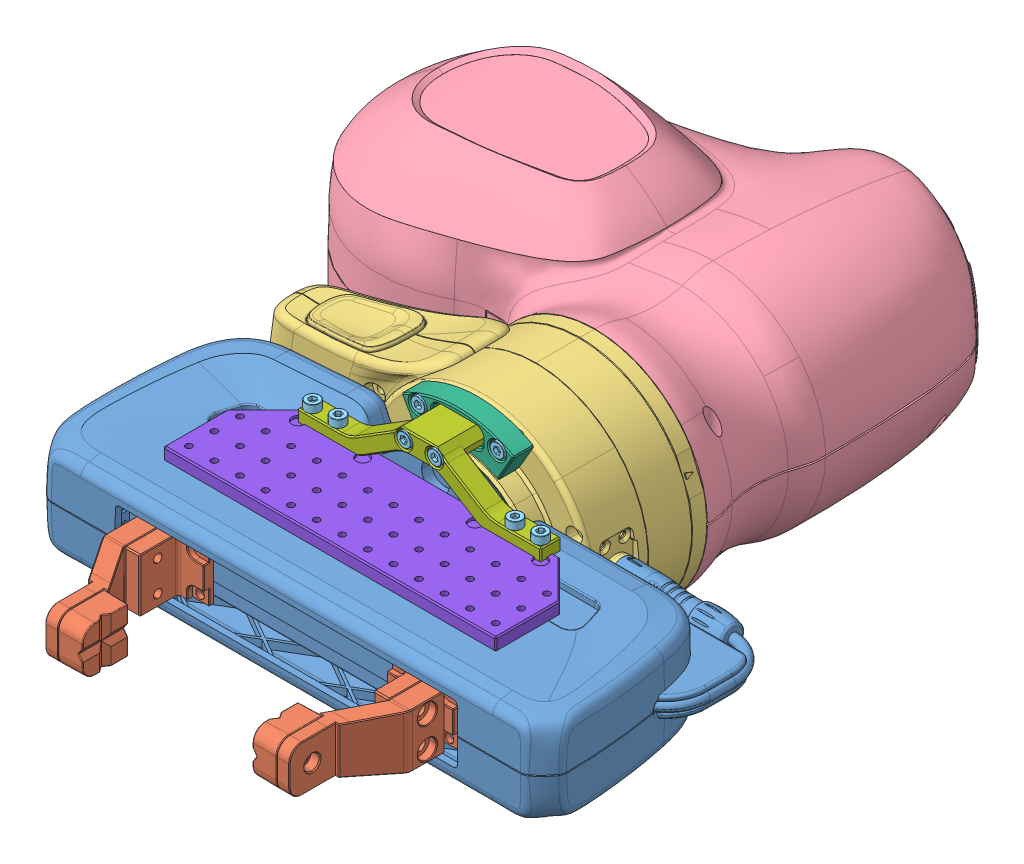
SolidWorks assembly FRANKA_wrist, configuration ﾃﾞﾌｫﾙﾄ. Lengths in mm.
Overall size (243.95 336.93 301.14).
28 component instances, 8 part files, 26 mates.
Components (placement in the parent):
- FRANKA_hand-1: FRANKA_hand [ﾃﾞﾌｫﾙﾄ] at (-106.4755 -4.1524 215.1453) size (209.36 63 139.58)
  - FRANKA_Hand_Standard^FRANKA_Hand_movable_Standard_FRANKA_including_FE_hand.STEP-1: FRANKA_Hand_Standard^FRANKA_Hand_movable_Standard_FRANKA_including_FE_hand.STEP [Default] at origin size (209.36 63 100.81)
  - FRANKA_Finger_Standard^FRANKA_Hand_movable_Standard_FRANKA_including_FE_hand.STEP-1: FRANKA_Finger_Standard^FRANKA_Hand_movable_Standard_FRANKA_including_FE_hand.STEP [Default] at (-31.2912 0 0) size (28.5 21 54)
  - FRANKA_Finger_Standard^FRANKA_Hand_movable_Standard_FRANKA_including_FE_hand.STEP-2: FRANKA_Finger_Standard^FRANKA_Hand_movable_Standard_FRANKA_including_FE_hand.STEP [Default] at (192.2912 0 0) x (-1 0 0) z (0 0 1) size (28.5 21 54)
- FRANKA_link7-1: FRANKA_link7 [Default] at (-25.9755 -4.152 59.7453) x (-0.707107 0.707107 0) z (-0.707107 -0.707107 0) size (143.77 55.46 143.77)
- FRANKA_link6-1: FRANKA_link6 [Default] at (-25.9755 -4.152 60.7453) x (1 0 0) z (0 1 0) size (211.94 250.58 301.08)
- hexagon socket head cap screw_jis-5: hexagon socket head cap screw_jis [JIS B 1176 M3 x 6 (6) --N] at (-70.5637 26.6633 177.7453) x (0 -1 0) z (-0.596742 0 0.802433) size (9 5.5 5.5)
- hexagon socket head cap screw_jis-6: hexagon socket head cap screw_jis [JIS B 1176 M3 x 6 (6) --N] at (-60.5637 26.6633 177.7453) x (0 -1 0) z (0.701533 0 0.712637) size (9 5.5 5.5)
- hexagon socket head cap screw_jis-7: hexagon socket head cap screw_jis [JIS B 1176 M3 x 6 (6) --N] at (-41.4526 33.2386 165.7453) x (0 0 -1) z (-0.153082 -0.988214 0) size (9 5.5 5.5)
- adapter-1-1: adapter-1 [Default] at (-106.4755 -4.1524 174.2453) size (43.5 16.47 8.35)
- adapter-2-1: adapter-2 [Default] at (-106.4755 -4.1524 163.7453) size (95.18 19.02 17.36)
- adapter-3-3: adapter-3 [Default] at (-106.4755 18.573 163.7453) x (-1 0 0) z (0 -1 0) size (130 40 5)
- hexagon socket head cap screw_jis-8: hexagon socket head cap screw_jis [JIS B 1176 M3 x 6 (6) --N] at (18.6126 26.6633 177.7453) x (0 -1 0) z (-0.596742 0 -0.802433) size (9 5.5 5.5)
- hexagon socket head cap screw_jis-9: hexagon socket head cap screw_jis [JIS B 1176 M3 x 6 (6) --N] at (8.6126 26.6633 177.7453) x (0 -1 0) z (0.701533 0 -0.712637) size (9 5.5 5.5)
- hexagon socket head cap screw_jis-10: hexagon socket head cap screw_jis [JIS B 1176 M3 x 6 (6) --N] at (-10.4985 33.2386 165.7453) x (0 0 -1) z (-0.153082 0.988214 0) size (9 5.5 5.5)
- hexagon socket head cap screw_jis-11: hexagon socket head cap screw_jis [JIS B 1176 M3 x 6 (6) --N] at (-70.5637 -34.9673 177.7453) x (0 1 0) z (0.596742 0 -0.802433) size (9 5.5 5.5)
- hexagon socket head cap screw_jis-12: hexagon socket head cap screw_jis [JIS B 1176 M3 x 6 (6) --N] at (-60.5637 -34.9673 177.7453) x (0 1 0) z (-0.701533 0 -0.712637) size (9 5.5 5.5)
- hexagon socket head cap screw_jis-13: hexagon socket head cap screw_jis [JIS B 1176 M3 x 6 (6) --N] at (-41.4526 -41.5426 165.7453) x (0 0 -1) z (0.153082 -0.988214 0) size (9 5.5 5.5)
- hexagon socket head cap screw_jis-14: hexagon socket head cap screw_jis [JIS B 1176 M3 x 6 (6) --N] at (18.6126 -34.9673 177.7453) x (0 1 0) z (0.596742 0 0.802433) size (9 5.5 5.5)
- hexagon socket head cap screw_jis-15: hexagon socket head cap screw_jis [JIS B 1176 M3 x 6 (6) --N] at (8.6126 -34.9673 177.7453) x (0 1 0) z (-0.701533 0 0.712637) size (9 5.5 5.5)
- hexagon socket head cap screw_jis-16: hexagon socket head cap screw_jis [JIS B 1176 M3 x 6 (6) --N] at (-10.4985 -41.5426 165.7453) x (0 0 -1) z (0.153082 0.988214 0) size (9 5.5 5.5)
- adapter-1-2: adapter-1 [Default] at (54.5245 -4.1516 174.2453) x (-1 0 0) z (0 0 1) size (43.5 16.47 8.35)
- adapter-2-2: adapter-2 [Default] at (54.5245 -4.1516 163.7453) x (-1 0 0) z (0 0 1) size (95.18 19.02 17.36)
- adapter-3-4: adapter-3 [Default] at (54.5245 -26.877 163.7453) x (1 0 0) z (0 1 0) size (130 40 5)
- hexagon socket head cap screw_jis-17: hexagon socket head cap screw_jis [JIS B 1176 M3 x 6 (6) --N] at (-31.9755 33.598 180.7453) x (0 0 -1) z (-0.633766 -0.773524 0) size (9 5.5 5.5)
- hexagon socket head cap screw_jis-18: hexagon socket head cap screw_jis [JIS B 1176 M3 x 6 (6) --N] at (-19.9755 33.598 180.7453) x (0 0 -1) z (-0.633766 0.773524 0) size (9 5.5 5.5)
- hexagon socket head cap screw_jis-19: hexagon socket head cap screw_jis [JIS B 1176 M3 x 6 (6) --N] at (-31.9755 -41.902 180.7453) x (0 0 -1) z (0.633766 -0.773524 0) size (9 5.5 5.5)
- hexagon socket head cap screw_jis-20: hexagon socket head cap screw_jis [JIS B 1176 M3 x 6 (6) --N] at (-19.9755 -41.902 180.7453) x (0 0 -1) z (0.633766 0.773524 0) size (9 5.5 5.5)
Mates (geometry in assembly coordinates):
- 同心円1: concentric: cylinder of FRANKA_link7-1 through (-43.6532 13.5257 166.7453) axis (0 0 1) radius 3; cylinder of FRANKA_hand-1/FRANKA_Hand_Standard^FRANKA_Hand_movable_Standard_FRANKA_including_FE_hand.STEP-1 through (-43.6532 13.5257 173.2453) axis (0 0 -1) radius 3
- 同心円2: concentric: cylinder of FRANKA_hand-1/FRANKA_Hand_Standard^FRANKA_Hand_movable_Standard_FRANKA_including_FE_hand.STEP-1 through (-25.9755 -4.152 164.2453) axis (0 0 1) radius 15.75; cylinder of FRANKA_link7-1 through (-25.9755 -4.152 99.2924) axis (0 0 -1) radius 15.75
- 同心円3: concentric: cylinder of FRANKA_link7-1 through (-25.9755 -4.152 52.4561) axis (0 0 -1) radius 44; cylinder of FRANKA_link6-1 through (-25.9755 -4.152 -5.2383) axis (0 0 -1) radius 33
- 一致2: coincident: plane of FRANKA_link7-1 through (-25.9755 -4.152 111.9453) normal (0 0 -1); plane of FRANKA_link6-1 through (-25.9755 -4.152 111.9453) normal (0 0 1)
- 平行1: parallel: plane of FRANKA_hand-1/FRANKA_Finger_Standard^FRANKA_Hand_movable_Standard_FRANKA_including_FE_hand.STEP-2 through (12.2579 -13.1527 279.1453) normal (0 -1 0); plane of FRANKA_link6-1 through (-113.9755 -18.952 60.7453) normal (0 -1 0)
- 相対固定1: in place: plane of FRANKA_hand-1/FRANKA_Hand_Standard^FRANKA_Hand_movable_Standard_FRANKA_including_FE_hand.STEP-1 through (-25.9755 -4.152 174.2453) normal (0 0 1); plane of ? through (0 0 174.2453) normal (0 0 1); moOrthogonalPlaneRef_w of FRANKA_hand-1/FRANKA_Hand_Standard^FRANKA_Hand_movable_Standard_FRANKA_including_FE_hand.STEP-1 through (-25.9755 -4.152 174.2453) normal (0 0 1); plane of ? through (0 0 174.2453) normal (0 1 0); plane of FRANKA_hand-1/FRANKA_Hand_Standard^FRANKA_Hand_movable_Standard_FRANKA_including_FE_hand.STEP-1 through (-25.9755 -4.152 174.2453) normal (0 0 1); plane of ? through (0 0 174.2453) normal (1 0 0); plane of FRANKA_hand-1/FRANKA_Hand_Standard^FRANKA_Hand_movable_Standard_FRANKA_including_FE_hand.STEP-1 through (-25.9755 -4.152 174.2453) normal (0 0 1); unknown of adapter-1-1
- 一致4: coincident: plane of FRANKA_hand-1/FRANKA_Hand_Standard^FRANKA_Hand_movable_Standard_FRANKA_including_FE_hand.STEP-1; plane of adapter-1-1
- 一致5: coincident: moOrthogonalPlaneRef_w of FRANKA_hand-1/FRANKA_Hand_Standard^FRANKA_Hand_movable_Standard_FRANKA_including_FE_hand.STEP-1 through (-106.4755 -4.1524 174.2453) normal (0 1 0); plane of adapter-1-1 through (-106.4755 -4.1524 174.2453) normal (0 1 0)
- 一致6: coincident: moOrthogonalPlaneRef_w of FRANKA_hand-1/FRANKA_Hand_Standard^FRANKA_Hand_movable_Standard_FRANKA_including_FE_hand.STEP-1 through (-106.4755 -4.1524 174.2453) normal (-1 0 0); plane of adapter-1-1 through (-106.4755 -4.1524 174.2453) normal (1 0 0)
- 一致7: coincident: plane of FRANKA_hand-1/FRANKA_Hand_Standard^FRANKA_Hand_movable_Standard_FRANKA_including_FE_hand.STEP-1 through (50.5245 10.848 166.7453) normal (0 0 -1); plane of FRANKA_link7-1 through (-14.8386 -15.2889 166.7453) normal (0 0 1)
- 相対固定2: in place: plane of adapter-1-1 through (-18.9755 34.598 163.7453) normal (0 0 1); plane of ? through (0 0 163.7453) normal (0 0 1); plane of adapter-1-1 through (-18.9755 34.598 163.7453) normal (0 0 1); plane of ? through (0 0 163.7453) normal (0 1 0); plane of adapter-1-1 through (-18.9755 34.598 163.7453) normal (0 0 1); plane of ? through (0 0 163.7453) normal (1 0 0); plane of adapter-1-1 through (-18.9755 34.598 163.7453) normal (0 0 1); unknown of adapter-2-1
- 一致8: coincident: plane of adapter-1-1; plane of adapter-2-1
- 一致9: coincident: moOrthogonalPlaneRef_w of adapter-1-1 through (-106.4755 -4.1524 163.7453) normal (0 1 0); plane of adapter-2-1 through (-106.4755 -4.1524 163.7453) normal (0 1 0)
- 一致10: coincident: moOrthogonalPlaneRef_w of adapter-1-1 through (-106.4755 -4.1524 163.7453) normal (-1 0 0); plane of adapter-2-1 through (-106.4755 -4.1524 163.7453) normal (1 0 0)
- 相対固定3: in place: plane of adapter-2-1 through (11.7064 17.573 175.7453) normal (0 -1 0); plane of ? through (0 17.573 0) normal (0 -1 0); plane of adapter-2-1 through (11.7064 17.573 175.7453) normal (0 -1 0); plane of ? through (0 17.573 0) normal (0 0 -1); plane of adapter-2-1 through (11.7064 17.573 175.7453) normal (0 -1 0); plane of ? through (0 17.573 0) normal (-1 0 0); plane of adapter-2-1 through (21.6126 18.573 172.7453) normal (0 -1 0); unknown of adapter-3-3
- 一致11: coincident: plane of adapter-2-1; plane of adapter-3-3
- 一致12: coincident: moOrthogonalPlaneRef_w of adapter-2-1 through (-106.4755 18.573 163.7453) normal (0 0 -1); plane of adapter-3-3 through (-106.4755 18.573 163.7453) normal (0 0 -1)
- 一致13: coincident: moOrthogonalPlaneRef_w of adapter-2-1 through (-106.4755 18.573 163.7453) normal (1 0 0); plane of adapter-3-3 through (-106.4755 18.573 163.7453) normal (-1 0 0)
- 同心円5: concentric: cylinder of adapter-2-1 through (-60.5637 23.6633 177.7453) axis (0 1 0) radius 1.6; cylinder of hexagon socket head cap screw_jis-6 through (-60.5637 58.4133 177.7453) axis (0 1 0) radius 1.5
- 一致15: coincident: plane of adapter-2-1 through (-53.5637 23.6633 172.7453) normal (0 1 0); plane of hexagon socket head cap screw_jis-6 through (-58.6039 23.6633 175.8161) normal (0 -1 0)
- 同心円6: concentric: cylinder of adapter-1-1 through (-41.4526 33.2386 165.7453) axis (0 0 1) radius 1.6; cylinder of hexagon socket head cap screw_jis-7 through (-41.4526 33.2386 197.4953) axis (0 0 1) radius 1.5
- 一致16: coincident: plane of adapter-1-1 through (-39.8526 33.2386 162.7453) normal (0 0 1); plane of hexagon socket head cap screw_jis-7 through (-38.735 32.8176 162.7453) normal (0 0 -1)
- 同心円7: concentric: cylinder of hexagon socket head cap screw_jis-5 through (-70.5637 58.4133 177.7453) axis (0 1 0) radius 1.5; cylinder of adapter-2-1 through (-70.5637 23.6633 177.7453) axis (0 1 0) radius 1.6
- 一致17: coincident: plane of hexagon socket head cap screw_jis-5 through (-68.357 23.6633 179.3864) normal (0 -1 0); plane of adapter-2-1 through (-53.5637 23.6633 172.7453) normal (0 1 0)
- 同心円9: concentric: circle of adapter-2-1; circle of hexagon socket head cap screw_jis-17
- 一致19: coincident: plane of adapter-2-1 through (-30.2755 33.598 177.7453) normal (0 0 1); plane of hexagon socket head cap screw_jis-17 through (-29.8484 31.8552 177.7453) normal (0 0 -1)
